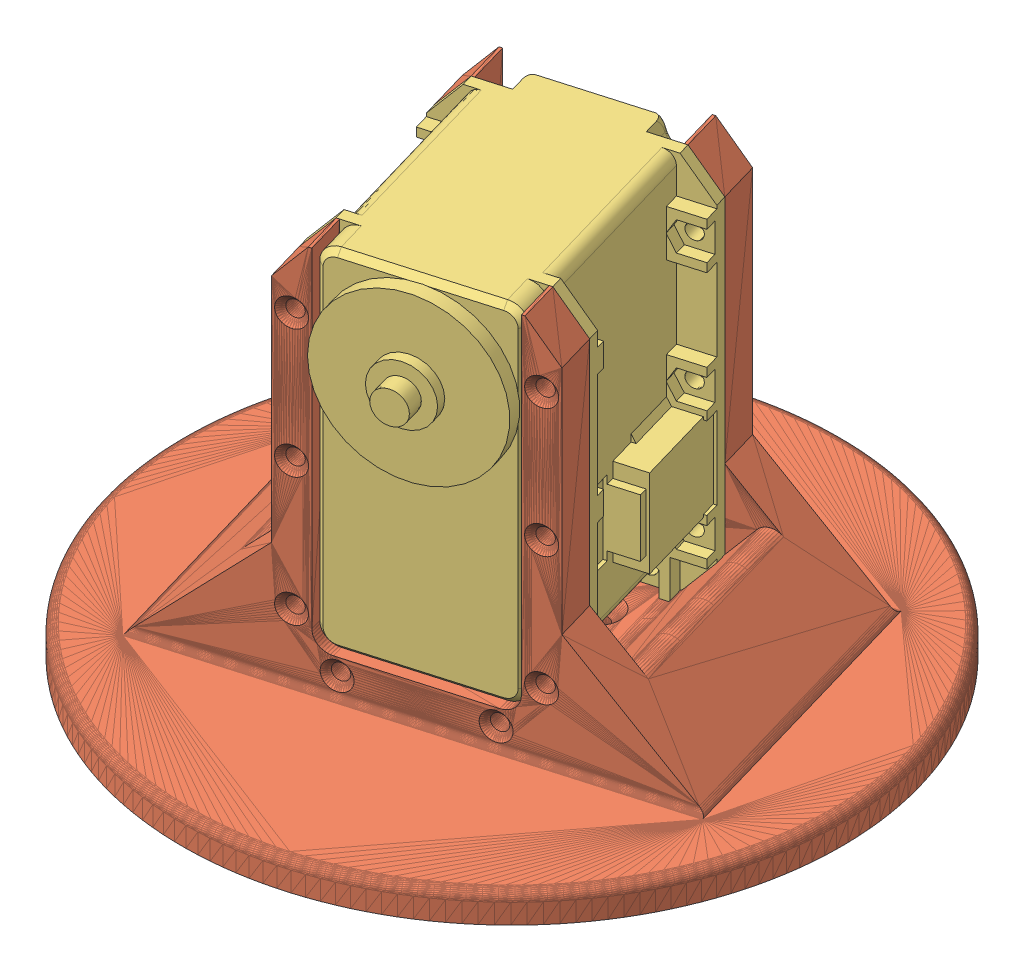
SolidWorks assembly Assem2, configuration Default. Lengths in mm.
Overall size (140.05 72.32 140.05).
3 component instances, 3 part files, 8 mates.
Components (placement in the parent):
- Base-disc-1: Base-disc [Default] at (40.5552 32.0167 101.6089) size (110 1 110)
- NewBase.step-1: NewBase.step [Default] at (40.6801 33.4506 101.0855) x (0.960222 0 -0.279236) z (0 1 0) size (112.99 113 71)
- MX-106T-1: MX-106T [Default] at (40.5074 89.0167 101.5981) x (0.960332 0 -0.27886) z (0.27886 0 0.960332) size (40.2 65.92 55.3)
Mates (geometry in assembly coordinates):
- Coincident8: coincident: plane of Base-disc-1 through (40.5552 33.0167 101.6089) normal (0 1 0); plane of NewBase.step-1 through (33.7072 33.0167 111.268) normal (0 -1 0)
- Concentric5: concentric: circle of Base-disc-1; circle of NewBase.step-1
- Coincident9: coincident: point of MX-106T-1; point of NewBase.step-1
- Coincident10: coincident: circle of MX-106T-1; point of NewBase.step-1
- Coincident11: coincident: circle of MX-106T-1; point of NewBase.step-1
- Coincident12: coincident: circle of MX-106T-1; point of NewBase.step-1
- Coincident13: coincident: circle of MX-106T-1; point of NewBase.step-1
- Coincident14: coincident: circle of MX-106T-1; point of NewBase.step-1
